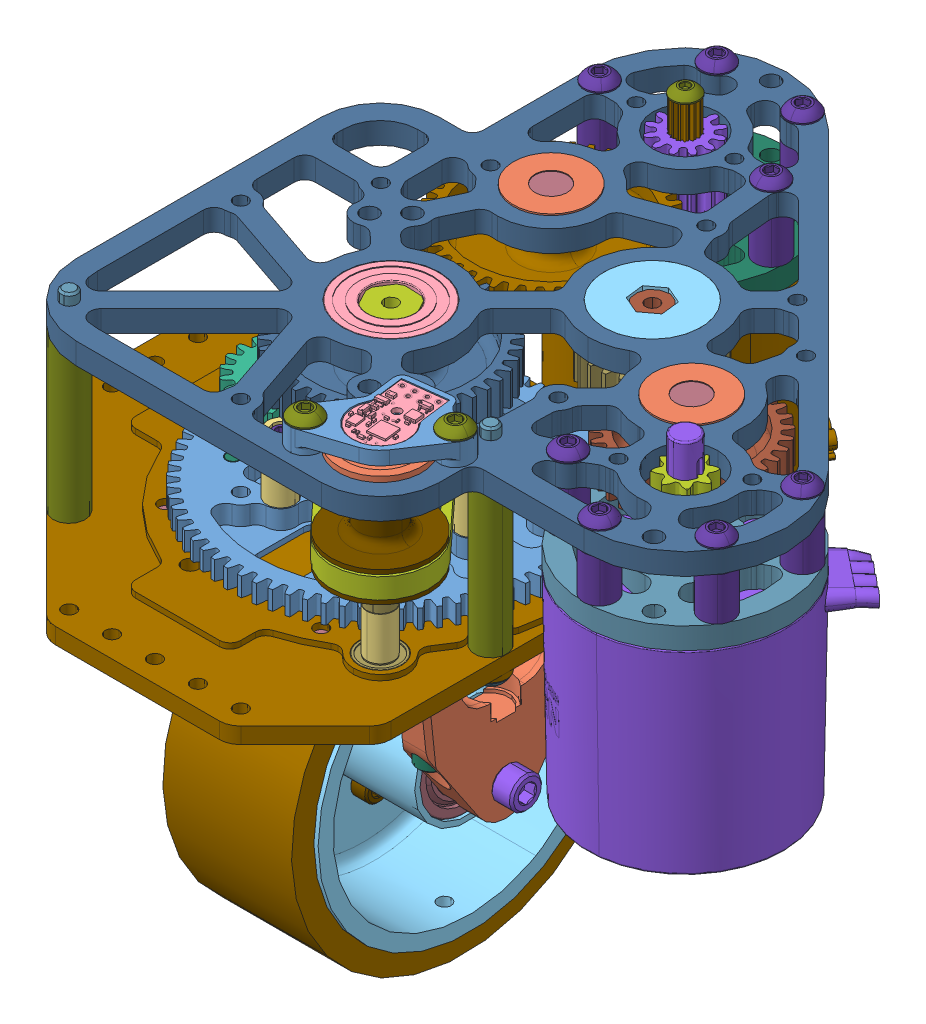
SolidWorks assembly WCP-0361 - Swerve X (Falcon Down, Neo Down) (WCP-0363), configuration Default. Lengths in mm.
Overall size (208.72 186.88 201.03).
107 component instances, 63 part files, 13 mates.
Components (placement in the parent):
- WCP-0361 - Swerve X (Tube Mount, Flipped Gears Below) (WCP-0363).step-1-1: WCP-0361 - Swerve X (Tube Mount, Flipped Gears Below) (WCP-0363).step-1 [Default] at origin size (208.72 184.42 201.03)
  - WCP-0364 Rev1 - WCP X Wheel Module.step-1-1: WCP-0364 Rev1 - WCP X Wheel Module.step-1 [Default] at (0 -0.825 0) size (95.62 174.54 137.74)
    - WCP-0364-001 Rev1.step-1-1: WCP-0364-001 Rev1.step-1 [Default] at (0 6.35 0) size (93.93 9.53 93.93)
    - WCP-0366 Rev1_Default_As Machined_.step-1-1: WCP-0366 Rev1_Default_As Machined_.step-1 [Default] at (29.2862 -49.2125 0) x (0 0 -1) z (1 0 0) size (51.81 60.46 9.5)
    - WCP-0366 Rev1_Default_As Machined_.step-1-2: WCP-0366 Rev1_Default_As Machined_.step-1 [Default] at (-29.2862 -49.2125 0) x (0 0 1) z (-1 0 0) size (51.81 60.46 9.5)
    - WCP-0364-006 Rev1.step-1-1: WCP-0364-006 Rev1.step-1 [Default] at (0 -49.2125 0) x (1 0 0) z (0 -0.837962 0.545729) size (56.46 12.67 12.67)
    - WCP-0364-005 Rev2.step-1-1: WCP-0364-005 Rev2.step-1 [Default] at (-29.2862 -1.2827 0) x (0 -1 0) z (0 0 1) size (54.08 11 11)
    - WCP-0365 Rev2.step-1-1: WCP-0365 Rev2.step-1 [Default] at (2.3061 -49.2125 0) x (0 -0.866025 -0.5) z (1 0 0) size (88.9 88.9 41.15)
    - WCP-0233 Rev1.step-1-1: WCP-0233 Rev1.step-1 [Default] at (-18.0375 -49.2125 0) x (0 0 -1) z (0 1 0) size (68.52 16.32 68.56)
    - WCP-0364-002 Rev1.step-1-1: WCP-0364-002 Rev1.step-1 [Default] at (0 34.5757 0) x (0 -1 0) z (0.999257 0 0.03854) size (51.69 15 15)
    - WCP-0276 Rev1.step-1-1: WCP-0276 Rev1.step-1 [Default] at (-29.2862 -15.4625 0) x (0 0 1) z (1 0 0) size (25.2 12.86 25.34)
    - WCP-0364-008 Rev1.step-1-1: WCP-0364-008 Rev1.step-1 [Default] at (2.3061 -49.2125 0) x (1 0 0) z (0 -0.879106 0.476626) size (38.1 101.6 101.6)
    - WCP-0357 Rev1.step-1-1: WCP-0357 Rev1.step-1 [Default] at origin size (88.91 6.35 88.9)
    - 217-5829_0375_flanged_thunderhex_bearing.step-1-1: 217-5829_0375_flanged_thunderhex_bearing.step-1 [Default] at (-29.2862 12.7 0) x (0 -1 0) z (0.06043 0 0.998172) size (7.11 24.61 24.61)
    - 217-3489_0_250_radial_bearing.step-1-1: 217-3489_0_250_radial_bearing.step-1 [Default] at (-29.2862 -29.3687 0) x (0 -1 0) z (0.460874 0 0.887465) size (4.76 12.7 12.7)
    - 217-3109_0_500_radial_bearing.step-1-1: 217-3109_0_500_radial_bearing.step-1 [Default] at (-17.8424 -49.2125 0) x (1 0 0) z (0 0.040496 0.99918) size (7.94 28.57 28.57)
    - 217-3109_0_500_radial_bearing.step-1-2: 217-3109_0_500_radial_bearing.step-1 [Default] at (18.0604 -49.2125 0) x (1 0 0) z (0 -0.205758 0.978603) size (7.94 28.57 28.57)
    - 217-2731_0_500_flanged_bearing.step-1-1: 217-2731_0_500_flanged_bearing.step-1 [Default] at (0 4.7625 0) x (0.999376 0 -0.035335) z (0.035335 0 0.999376) size (31.12 7.94 31.12)
    - NFS-0018_SHCS_#10-32_1_750L_Default_As Machined_.step-1-1: NFS-0018_SHCS_#10-32_1_750L_Default_As Machined_.step-1 [Default] at (-29.2862 11.1125 17.4625) x (0.988526 0 -0.151053) z (0 1 0) size (7.92 7.92 49.28)
    - NFS-0018_SHCS_#10-32_1_750L_Default_As Machined_.step-1-2: NFS-0018_SHCS_#10-32_1_750L_Default_As Machined_.step-1 [Default] at (-29.2862 11.1125 -17.4625) x (0.988526 0 -0.151053) z (0 1 0) size (7.92 7.92 49.28)
    - NFS-0018_SHCS_#10-32_1_750L_Default_As Machined_.step-1-3: NFS-0018_SHCS_#10-32_1_750L_Default_As Machined_.step-1 [Default] at (29.2862 11.1125 17.4625) x (0.988526 0 -0.151053) z (0 1 0) size (7.92 7.92 49.28)
    - NFS-0018_SHCS_#10-32_1_750L_Default_As Machined_.step-1-4: NFS-0018_SHCS_#10-32_1_750L_Default_As Machined_.step-1 [Default] at (29.2862 11.1125 -17.4625) x (0.988526 0 -0.151053) z (0 1 0) size (7.92 7.92 49.28)
    - 8-32 BHCS_0.500.step-1-1: 8-32 BHCS_0.500.step-1 [Default] at (-29.2862 23.8633 0) x (0.940105 0 -0.340884) z (0.340884 0 0.940105) size (7.92 14.92 7.92)
    - NFS-0059_SHCS_#4-40_0_875L_91251A113.step-1-1: NFS-0059_SHCS_#4-40_0_875L_91251A113.step-1 [Default] at (23.876 3.5687 0) x (0.431119 0 0.902295) z (0 -1 0) size (4.65 4.65 25.08)
    - NFS-0059_SHCS_#4-40_0_875L_91251A113.step-1-2: NFS-0059_SHCS_#4-40_0_875L_91251A113.step-1 [Default] at (23.876 3.0654 0) x (0.520663 0 0.853762) z (0 -1 0) size (4.65 4.65 25.08)
    - NFS-0059_SHCS_#4-40_0_875L_91251A113.step-1-3: NFS-0059_SHCS_#4-40_0_875L_91251A113.step-1 [Default] at (-11.938 3.5687 -20.6772) x (0.431119 0 0.902295) z (0 -1 0) size (4.65 4.65 25.08)
    - NFS-0059_SHCS_#4-40_0_875L_91251A113.step-1-4: NFS-0059_SHCS_#4-40_0_875L_91251A113.step-1 [Default] at (-11.938 3.0654 -20.6772) x (0.520663 0 0.853762) z (0 -1 0) size (4.65 4.65 25.08)
    - NFS-0059_SHCS_#4-40_0_875L_91251A113.step-1-5: NFS-0059_SHCS_#4-40_0_875L_91251A113.step-1 [Default] at (-11.938 3.0654 20.6772) x (0.520663 0 0.853762) z (0 -1 0) size (4.65 4.65 25.08)
    - 10-32 SHCS - No Thread_WCP-0265 - 0.375.step-1-1: 10-32 SHCS - No Thread_WCP-0265 - 0.375.step-1 [Default] at (-8.2862 -59.5312 17.8726) x (0 -0.796051 -0.60523) z (0 -0.60523 0.796051) size (7.67 14.35 7.67)
    - 10-32 SHCS - No Thread_WCP-0265 - 0.375.step-1-2: 10-32 SHCS - No Thread_WCP-0265 - 0.375.step-1 [Default] at (-8.2862 -38.8937 -17.8726) x (0 -0.796051 -0.60523) z (0 -0.60523 0.796051) size (7.67 14.35 7.67)
    - 10-32 SHCS - No Thread_WCP-0265 - 0.375.step-1-3: 10-32 SHCS - No Thread_WCP-0265 - 0.375.step-1 [Default] at (-8.2862 -38.8937 17.8726) x (0 -0.796051 -0.60523) z (0 -0.60523 0.796051) size (7.67 14.35 7.67)
    - 10-32 SHCS - No Thread_WCP-0265 - 0.375.step-1-4: 10-32 SHCS - No Thread_WCP-0265 - 0.375.step-1 [Default] at (-8.2862 -59.5312 -17.8726) x (0 -0.796051 -0.60523) z (0 -0.60523 0.796051) size (7.67 14.35 7.67)
    - 10-32 SHCS - No Thread_WCP-0265 - 0.375.step-1-5: 10-32 SHCS - No Thread_WCP-0265 - 0.375.step-1 [Default] at (-8.2862 -28.575 0) x (0 -0.796051 -0.60523) z (0 -0.60523 0.796051) size (7.67 14.35 7.67)
    - 10-32 SHCS - No Thread_WCP-0265 - 0.375.step-1-6: 10-32 SHCS - No Thread_WCP-0265 - 0.375.step-1 [Default] at (-8.2862 -69.85 0) x (0 0.591573 -0.806252) z (0 -0.806252 -0.591573) size (7.67 14.35 7.67)
    - NFS-0024_250-20_thin_locknut_90566A029.step-1-1: NFS-0024_250-20_thin_locknut_90566A029.step-1 [Default] at (-34.0362 -49.2125 0) x (0 0.824738 0.565516) z (0 -0.565516 0.824738) size (11.14 5.19 12.86)
    - WCP-0229 Rev1.step-1-1: WCP-0229 Rev1.step-1 [Default] at (-22.6822 -49.2125 0) size (0.89 16.1 14.34)
    - WCP-0229 Rev1.step-1-2: WCP-0229 Rev1.step-1 [Default] at (22.6822 -49.2125 0) size (0.89 16.1 14.34)
    - WCP-0367-002 Rev3.step-1-1: WCP-0367-002 Rev3.step-1 [Default] at (0 28.6559 0) x (0 0 -1) z (1 0 0) size (49.74 26.04 44.2)
    - WCP-0367-006 Rev1.step-1-1: WCP-0367-006 Rev1.step-1 [Default] at (-29.2862 -3.81 0) size (17.27 17.14 17.27)
    - WCP-0367-010 Rev1.step-1-1: WCP-0367-010 Rev1.step-1 [Default] at (-29.2862 22.2758 0) x (0 0 1) z (-1 0 0) size (12.7 4.76 12.7)
    - WCP-0434 Rev1.step-1-1: WCP-0434 Rev1.step-1 [Default] at (-29.2862 19 0) x (-0.327758 0 -0.944762) z (0 -1 0) size (30.3 30.48 12.6)
    - 217-5464_24T_500_hex_steel.step-1-1: 217-5464_24T_500_hex_steel.step-1 [Default] at (0 19 0) x (0.428371 0 0.903603) z (0 -1 0) size (32.87 32.87 12.6)
    - 0250-20_3L_SHCS_91251A554.step-1-1: 0250-20_3L_SHCS_91251A554.step-1 [Default] at (-0.8888 -49.2125 0) x (0 -0.133483 -0.991051) z (1 0 0) size (9.53 9.53 82.55)
  - 217-3489_0_250_radial_bearing.step-1-1: 217-3489_0_250_radial_bearing.step-1 [Default] at (36.5633 1.6187 39.7383) x (0 1 0) z (-0.269707 0 0.962942) size (4.76 12.7 12.7)
  - WCP-0360-001 Rev1.step-1-1: WCP-0360-001 Rev1.step-1 [Default] at origin size (133.35 8 133.35)
  - WCP-0361-001 Rev2.step-1-1: WCP-0361-001 Rev2.step-1 [Default] at (0 53.1812 0) size (174.12 6.35 174.12)
  - WCP-0364-003 Rev1.step-1-1: WCP-0364-003 Rev1.step-1 [Default] at (38.669 7.5147 -38.669) x (0.682654 0 0.730742) z (0 1 0) size (20.01 20.32 56.54)
  - WCP-0364-004 Rev1.step-1-1: WCP-0364-004 Rev1.step-1 [Default] at (36.5633 23.984 39.7383) x (0 1 0) z (-0.373833 0 -0.927496) size (58.72 11 11)
  - WCP-0361-004 Rev1_Default_As Machined_.step-1-1: WCP-0361-004 Rev1_Default_As Machined_.step-1 [Default] at (69.0125 43.1356 -19.9819) x (0 -1 0) z (-0.01804 0 -0.999837) size (25.16 11 11)
  - WCP-0361-004 Rev1_Default_As Machined_.step-1-2: WCP-0361-004 Rev1_Default_As Machined_.step-1 [Default] at (-5.7166 43.1356 -53.1094) x (0 -1 0) z (0.932067 0 0.362285) size (25.16 11 11)
  - WCP-0361-005 Rev1.step-1-1: WCP-0361-005 Rev1.step-1 [Default] at (86.9695 34.1313 -0.16) x (0.741112 0 -0.671382) z (0.671382 0 0.741112) size (60 6.35 71.67)
  - WCP-0361-002 Rev1.step-1-1: WCP-0361-002 Rev1.step-1 [Default] at (0.16 34.1313 -86.9695) x (-0.985271 0 -0.170999) z (0.170999 0 -0.985271) size (60 6.35 79.29)
  - WCP-0387 Rev1.step-1-1: WCP-0387 Rev1.step-1 [Default] at (49.2125 26.1937 19.7361) x (0 -1 0) z (0.97467 0 0.223647) size (47.62 9.5 9.5)
  - WCP-0387 Rev1.step-1-2: WCP-0387 Rev1.step-1 [Default] at (-47.625 26.1937 47.625) x (0 -1 0) z (-0.427741 0 0.903901) size (47.62 9.5 9.5)
  - WCP-0202 Rev1.step-1-1: WCP-0202 Rev1.step-1 [Default] at (-12.54 43.6562 -108.9665) x (0 -1 0) z (0.721842 0 0.692058) size (12.7 9.5 9.5)
  - WCP-0202 Rev1.step-1-2: WCP-0202 Rev1.step-1 [Default] at (108.9665 43.6562 -12.86) x (0 -1 0) z (0.721842 0 0.692058) size (12.7 9.5 9.5)
  - WCP-0202 Rev1.step-1-3: WCP-0202 Rev1.step-1 [Default] at (64.9724 43.6562 12.54) x (0 -1 0) z (0.721842 0 0.692058) size (12.7 9.5 9.5)
  - WCP-0202 Rev1.step-1-4: WCP-0202 Rev1.step-1 [Default] at (25.56 43.6562 -86.9695) x (0 -1 0) z (0.721842 0 0.692058) size (12.7 9.5 9.5)
  - WCP-0202 Rev1.step-1-5: WCP-0202 Rev1.step-1 [Default] at (86.9695 43.6562 25.24) x (0 -1 0) z (0.721842 0 0.692058) size (12.7 9.5 9.5)
  - WCP-0202 Rev1.step-1-6: WCP-0202 Rev1.step-1 [Default] at (-25.24 43.6562 -86.9695) x (0 -1 0) z (0.721842 0 0.692058) size (12.7 9.5 9.5)
  - WCP-0202 Rev1.step-1-7: WCP-0202 Rev1.step-1 [Default] at (12.86 43.6562 -108.9665) x (0 -1 0) z (0.721842 0 0.692058) size (12.7 9.5 9.5)
  - WCP-0202 Rev1.step-1-8: WCP-0202 Rev1.step-1 [Default] at (108.9665 43.6562 12.54) x (0 -1 0) z (0.721842 0 0.692058) size (12.7 9.5 9.5)
  - WCP-0226 Rev1.step-1-1: WCP-0226 Rev1.step-1 [Default] at (-19.7361 16.6687 -49.2125) x (0 1 0) z (0.900957 0 0.433909) size (28.57 9.5 9.5)
  - WCP-0307 Rev1.step-1-1: WCP-0307 Rev1.step-1 [Default] at (-19.7361 -5.5913 -49.2125) x (0 -1 0) z (-0.403935 0 0.914788) size (3.18 9.5 9.5)
  - 217-2733_0_375_flanged_bearing.step-1-1: 217-2733_0_375_flanged_bearing.step-1 [Default] at (69.0125 49.6887 -19.9819) x (0 1 0) z (0.053261 0 -0.998581) size (7.11 24.61 24.61)
  - 217-2733_0_375_flanged_bearing.step-1-2: 217-2733_0_375_flanged_bearing.step-1 [Default] at (36.5633 57.9438 39.7383) x (0 -1 0) z (0.710471 0 -0.703726) size (7.11 24.61 24.61)
  - 217-2733_0_375_flanged_bearing.step-1-3: 217-2733_0_375_flanged_bearing.step-1 [Default] at (-5.7166 49.6887 -53.1094) x (0 1 0) z (0.053261 0 -0.998581) size (7.11 24.61 24.61)
  - WCP-0041_0_250_radial_bearing.step-1-1: WCP-0041_0_250_radial_bearing.step-1 [Default] at (38.669 1.5108 -38.669) x (-0.316483 0 0.948598) z (0 -1 0) size (15.88 15.88 4.98)
  - 217-4006_0_500_flanged_thunderhex_bearing.step-1-1: 217-4006_0_500_flanged_thunderhex_bearing.step-1 [Default] at (0 52.3875 0) x (-0.903668 0 0.428233) z (0 -1 0) size (31.12 31.12 7.94)
  - 217-2735_0_375_flanged_hex_bearing.step-1-1: 217-2735_0_375_flanged_hex_bearing.step-1 [Default] at (38.669 56.3562 -38.669) x (-0.91814 0 -0.396256) z (-0.396256 0 0.91814) size (31.12 7.94 31.12)
  - WCP-0042_0_250_flanged_bearing.step-1-1: WCP-0042_0_250_flanged_bearing.step-1 [Default] at (69.0125 33.8899 -19.9819) x (0.753109 0 -0.657896) z (0 1 0) size (18.24 18.24 4.98)
  - WCP-0042_0_250_flanged_bearing.step-1-2: WCP-0042_0_250_flanged_bearing.step-1 [Default] at (-5.7166 33.8899 -53.1094) x (0.890667 0 -0.454657) z (0 1 0) size (18.24 18.24 4.98)
  - 217-6915_Falcon_8T.step-1-1: 217-6915_Falcon_8T.step-1 [Default] at (86.9695 46.7088 -0.16) x (0.340812 0 -0.940132) z (0 -1 0) size (13.62 13.62 19.06)
  - 217-6919_Falcon_12T.step-1-1: 217-6919_Falcon_12T.step-1 [Default] at (0.16 46.7088 -86.9695) x (-0.557793 0 0.82998) z (0 -1 0) size (17.78 17.78 19.05)
  - WCP-0541 Rev1.step-1-1: WCP-0541 Rev1.step-1 [Default] at (-5.7166 43.1482 -53.1094) x (0.992001 0 0.126228) z (0 1 0) size (55.8 55.88 12.65)
  - WCP-0178 Rev1.step-1-1: WCP-0178 Rev1.step-1 [Default] at (0 42.0941 0) x (0.993242 0 -0.116064) z (0 1 0) size (55.8 55.88 12.65)
  - WCP-0540 Rev1.step-1-1: WCP-0540 Rev1.step-1 [Default] at (69.0125 43.1236 -19.9819) x (0.992415 0 -0.122933) z (0 1 0) size (43.07 43.07 12.6)
  - WCP-0538 Rev1.step-1-1: WCP-0538 Rev1.step-1 [Default] at (38.669 41.9158 -38.669) x (0.27049 0 -0.962723) z (0 1 0) size (32.86 32.86 12.65)
  - 10-32 BHCS - No Thread_WCP-0251 - 0.250.step-1-1: 10-32 BHCS - No Thread_WCP-0251 - 0.250.step-1 [Default] at (-33.4155 -4 33.4155) x (0.140263 0 -0.990114) z (-0.990114 0 -0.140263) size (9.17 8.92 9.17)
  - 10-32 BHCS - No Thread_WCP-0251 - 0.250.step-1-2: 10-32 BHCS - No Thread_WCP-0251 - 0.250.step-1 [Default] at (7.3926 -4 -46.6749) x (0.4685 0 0.883464) z (0.883464 0 -0.4685) size (9.17 8.92 9.17)
  - 10-32 BHCS - No Thread_WCP-0251 - 0.250.step-1-3: 10-32 BHCS - No Thread_WCP-0251 - 0.250.step-1 [Default] at (46.6749 -4 -7.3926) x (-0.69545 0 0.718575) z (0.718575 0 0.69545) size (9.17 8.92 9.17)
  - 10-32 BHCS - No Thread_WCP-0251 - 0.250.step-1-4: 10-32 BHCS - No Thread_WCP-0251 - 0.250.step-1 [Default] at (-42.106 -4 -21.4541) x (0.984998 0 -0.172564) z (-0.172564 0 -0.984998) size (9.17 8.92 9.17)
  - 10-32 BHCS - No Thread_WCP-0251 - 0.250.step-1-5: 10-32 BHCS - No Thread_WCP-0251 - 0.250.step-1 [Default] at (21.4541 -4 42.106) x (-0.898311 0 -0.43936) z (-0.43936 0 0.898311) size (9.17 8.92 9.17)
  - 10-32 BHCS - No Thread_WCP-0261 - 2.500.step-1-1: 10-32 BHCS - No Thread_WCP-0261 - 2.500.step-1 [Default] at (49.2125 -4 19.7361) x (0.670106 0 -0.742266) z (-0.742266 0 -0.670106) size (9.17 66.07 9.17)
  - 10-32 BHCS - No Thread_WCP-0261 - 2.500.step-1-2: 10-32 BHCS - No Thread_WCP-0261 - 2.500.step-1 [Default] at (-47.625 -4 47.625) x (0.958479 0 -0.285162) z (-0.285162 0 -0.958479) size (9.17 66.07 9.17)
  - 10-32 BHCS - No Thread_WCP-0258 - 1.750.step-1-1: 10-32 BHCS - No Thread_WCP-0258 - 1.750.step-1 [Default] at (-19.7361 -7.175 -49.2125) x (0.978856 0 -0.204553) z (-0.204553 0 -0.978856) size (9.17 47.02 9.17)
  - 10-32 BHCS - No Thread_WCP-0253 - 0.500.step-1-1: 10-32 BHCS - No Thread_WCP-0253 - 0.500.step-1 [Default] at (23.914 62.9348 49.3306) x (-0.153016 0 -0.988224) z (0.988224 0 -0.153016) size (9.17 15.27 9.17)
  - 10-32 BHCS - No Thread_WCP-0253 - 0.500.step-1-2: 10-32 BHCS - No Thread_WCP-0253 - 0.500.step-1 [Default] at (49.2125 62.9348 30.146) x (0.162273 0 -0.986746) z (0.986746 0 0.162273) size (9.17 15.27 9.17)
  - 10-32 BHCS - No Thread_WCP-0256 - 1.250.step-1-1: 10-32 BHCS - No Thread_WCP-0256 - 1.250.step-1 [Default] at (64.9724 56.3562 12.54) x (0.165498 0 -0.98621) z (0.98621 0 0.165498) size (9.17 34.32 9.17)
  - 10-32 BHCS - No Thread_WCP-0256 - 1.250.step-1-2: 10-32 BHCS - No Thread_WCP-0256 - 1.250.step-1 [Default] at (86.9695 56.3562 25.24) x (0.162273 0 -0.986746) z (0.986746 0 0.162273) size (9.17 34.32 9.17)
  - 10-32 BHCS - No Thread_WCP-0256 - 1.250.step-1-6: 10-32 BHCS - No Thread_WCP-0256 - 1.250.step-1 [Default] at (108.9665 56.3562 -12.86) x (-0.767084 0 0.641546) z (-0.641546 0 -0.767084) size (9.17 34.32 9.17)
  - 10-32 BHCS - No Thread_WCP-0256 - 1.250.step-1-7: 10-32 BHCS - No Thread_WCP-0256 - 1.250.step-1 [Default] at (108.9665 56.3562 12.54) x (0.162273 0 -0.986746) z (0.986746 0 0.162273) size (9.17 34.32 9.17)
  - WCP-0367-003 Rev2.step-1-1: WCP-0367-003 Rev2.step-1 [Default] at (36.5633 25.8309 39.7383) x (-0.999998 0 0.001857) z (0 -1 0) size (29.05 29.05 26.83)
  - WCP-0367-012 Rev1_30 Left.step-1-1: WCP-0367-012 Rev1_30 Left.step-1 [Default] at (36.5633 60.9155 39.7383) x (-0.992171 0 0.124885) z (-0.124885 0 -0.992171) size (37.02 6.58 29.76)
  - WCP-0367-001 Rev1.step-1-1: WCP-0367-001 Rev1.step-1 [Default] at (0 35.3446 0) x (0.987744 0 0.156082) z (-0.156082 0 0.987744) size (19.05 0.51 19.05)
  - WCP-0367-004 Rev1.step-1-1: WCP-0367-004 Rev1.step-1 [Default] at (36.5633 10.35 39.7383) size (8 12.7 8)
  - CANcoder.step-1-1: CANcoder.step-1 [Default] at (36.5485 59.1546 39.7225) x (-0.992171 0 0.124885) z (0 1 0) size (15.94 23.28 4.54)
  - WCP-0156 Rev1.step-1-1: WCP-0156 Rev1.step-1 [Default] at (36.5633 51.5938 39.7383) size (6.35 12.7 6.35)
  - Falcon_Motor_Spacer_0625.step-1-2: Falcon_Motor_Spacer_0625.step-1 [Default] at (86.9695 36.39 -0.16) size (12.7 1.59 12.7)
  - Encoder Belt.step-1-1: Encoder Belt.step-1 [Default] at (18.2816 30.8309 19.8691) x (0.677097 0 0.735894) z (-0.735894 0 0.677097) size (83.28 6 29.28)
- NEO Motor (REV-21-1650)-1-1: NEO Motor (REV-21-1650)-1 [Default] at (86.9695 30.9563 -0.16) x (0.113772 0 0.993507) z (0 1 0) size (65.4 64.76 93.26)
- 217-6515_Falcon_500_Default_As Machined_.step-1-1: 217-6515_Falcon_500_Default_As Machined_.step-1 [Default] at (0.16 4.7562 -86.9695) x (1 0 0) z (0 1 0) size (60 60 115.81)
- 8-32 BHCS_0.500.step-1-1: 8-32 BHCS_0.500.step-1 [Default] at (0.16 65.7588 -86.9695) x (-0.947071 0 0.321024) z (-0.321024 0 -0.947071) size (7.92 14.92 7.92)
- 10-32 BHCS - No Thread_WCP-0256 - 1.250.step-1-2: 10-32 BHCS - No Thread_WCP-0256 - 1.250.step-1 [Default] at (25.56 56.3562 -86.9695) x (-1 0 0) z (0 0 -1) size (9.17 34.32 9.17)
- 10-32 BHCS - No Thread_WCP-0256 - 1.250.step-1-10: 10-32 BHCS - No Thread_WCP-0256 - 1.250.step-1 [Default] at (12.86 56.3562 -108.9665) x (-0.982082 0 0.188455) z (-0.188455 0 -0.982082) size (9.17 34.32 9.17)
- 10-32 BHCS - No Thread_WCP-0256 - 1.250.step-1-14: 10-32 BHCS - No Thread_WCP-0256 - 1.250.step-1 [Default] at (-12.54 56.3562 -108.9665) x (-0.8 0 0.6) z (-0.6 0 -0.8) size (9.17 34.32 9.17)
- 10-32 BHCS - No Thread_WCP-0256 - 1.250.step-1-16: 10-32 BHCS - No Thread_WCP-0256 - 1.250.step-1 [Default] at (-25.24 56.3562 -86.9695) x (-0.63358 0 0.773678) z (-0.773678 0 -0.63358) size (9.17 34.32 9.17)
Mates (geometry in assembly coordinates):
- Coincident1: coincident anti-aligned: plane of WCP-0361 - Swerve X (Tube Mount, Flipped Gears Below) (WCP-0363).step-1-1/WCP-0361-002 Rev1.step-1-1 through (0.16 30.9563 -86.9695) normal (0 -1 0); plane of 217-6515_Falcon_500_Default_As Machined_.step-1-1 through (0.16 30.9563 -86.9695) normal (0 1 0)
- Concentric1: concentric aligned: cylinder of WCP-0361 - Swerve X (Tube Mount, Flipped Gears Below) (WCP-0363).step-1-1/WCP-0361-001 Rev2.step-1-1 through (0.16 -196.2358 -86.9695) axis (0 1 0) radius 9.5885; cylinder of 217-6515_Falcon_500_Default_As Machined_.step-1-1 through (0.16 65.7588 -86.9695) axis (0 1 0) radius 1.7272
- Concentric3: concentric aligned: cylinder of 217-6515_Falcon_500_Default_As Machined_.step-1-1 through (0.16 65.7588 -86.9695) axis (0 1 0) radius 1.7272; cylinder of 8-32 BHCS_0.500.step-1-1 through (0.16 67.9686 -86.9695) axis (0 1 0) radius 3.9624
- Coincident6: coincident anti-aligned: plane of 217-6515_Falcon_500_Default_As Machined_.step-1-1 through (0.16 65.7588 -86.9695) normal (0 1 0); plane of 8-32 BHCS_0.500.step-1-1 through (0.16 65.7588 -86.9695) normal (0 -1 0)
- Concentric4: concentric aligned: cylinder of WCP-0361 - Swerve X (Tube Mount, Flipped Gears Below) (WCP-0363).step-1-1/WCP-0361-002 Rev1.step-1-1 through (25.56 30.9563 -86.9695) axis (0 1 0) radius 2.4892; cylinder of 10-32 BHCS - No Thread_WCP-0256 - 1.250.step-1-2 through (25.56 24.6062 -86.9695) axis (0 1 0) radius 2.3749
- Coincident7: coincident anti-aligned: plane of WCP-0361 - Swerve X (Tube Mount, Flipped Gears Below) (WCP-0363).step-1-1/WCP-0361-001 Rev2.step-1-1 through (0 56.3562 0) normal (0 1 0); plane of 10-32 BHCS - No Thread_WCP-0256 - 1.250.step-1-2 through (25.56 56.3562 -86.9695) normal (0 -1 0)
- Concentric9: concentric aligned: cylinder of WCP-0361 - Swerve X (Tube Mount, Flipped Gears Below) (WCP-0363).step-1-1/WCP-0361-001 Rev2.step-1-1 through (12.86 50.0063 -108.9665) axis (0 1 0) radius 2.4892; cylinder of 217-6515_Falcon_500_Default_As Machined_.step-1-1 through (12.86 28.4163 -108.9665) axis (0 1 0) radius 2.0193
- Concentric10: concentric aligned: cylinder of WCP-0361 - Swerve X (Tube Mount, Flipped Gears Below) (WCP-0363).step-1-1/WCP-0361-001 Rev2.step-1-1 through (12.86 50.0063 -108.9665) axis (0 1 0) radius 2.4892; cylinder of 10-32 BHCS - No Thread_WCP-0256 - 1.250.step-1-10 through (12.86 24.6062 -108.9665) axis (0 1 0) radius 2.3749
- Coincident8: coincident anti-aligned: plane of WCP-0361 - Swerve X (Tube Mount, Flipped Gears Below) (WCP-0363).step-1-1/WCP-0361-001 Rev2.step-1-1 through (0 56.3562 0) normal (0 1 0); plane of 10-32 BHCS - No Thread_WCP-0256 - 1.250.step-1-10 through (12.86 56.3562 -108.9665) normal (0 -1 0)
- Concentric12: concentric aligned: cylinder of WCP-0361 - Swerve X (Tube Mount, Flipped Gears Below) (WCP-0363).step-1-1/WCP-0361-001 Rev2.step-1-1 through (-12.54 50.0063 -108.9665) axis (0 1 0) radius 2.4892; cylinder of 10-32 BHCS - No Thread_WCP-0256 - 1.250.step-1-14 through (-12.54 24.6062 -108.9665) axis (0 1 0) radius 2.3749
- Coincident10: coincident anti-aligned: plane of WCP-0361 - Swerve X (Tube Mount, Flipped Gears Below) (WCP-0363).step-1-1/WCP-0361-001 Rev2.step-1-1 through (0 56.3562 0) normal (0 1 0); plane of 10-32 BHCS - No Thread_WCP-0256 - 1.250.step-1-14 through (-12.54 56.3562 -108.9665) normal (0 -1 0)
- Concentric13: concentric aligned: cylinder of WCP-0361 - Swerve X (Tube Mount, Flipped Gears Below) (WCP-0363).step-1-1/WCP-0361-001 Rev2.step-1-1 through (-25.24 50.0063 -86.9695) axis (0 1 0) radius 2.4892; cylinder of 10-32 BHCS - No Thread_WCP-0256 - 1.250.step-1-16 through (-25.24 24.6062 -86.9695) axis (0 1 0) radius 2.3749
- Coincident11: coincident anti-aligned: plane of WCP-0361 - Swerve X (Tube Mount, Flipped Gears Below) (WCP-0363).step-1-1/WCP-0361-001 Rev2.step-1-1 through (0 56.3562 0) normal (0 1 0); plane of 10-32 BHCS - No Thread_WCP-0256 - 1.250.step-1-16 through (-25.24 56.3562 -86.9695) normal (0 -1 0)
